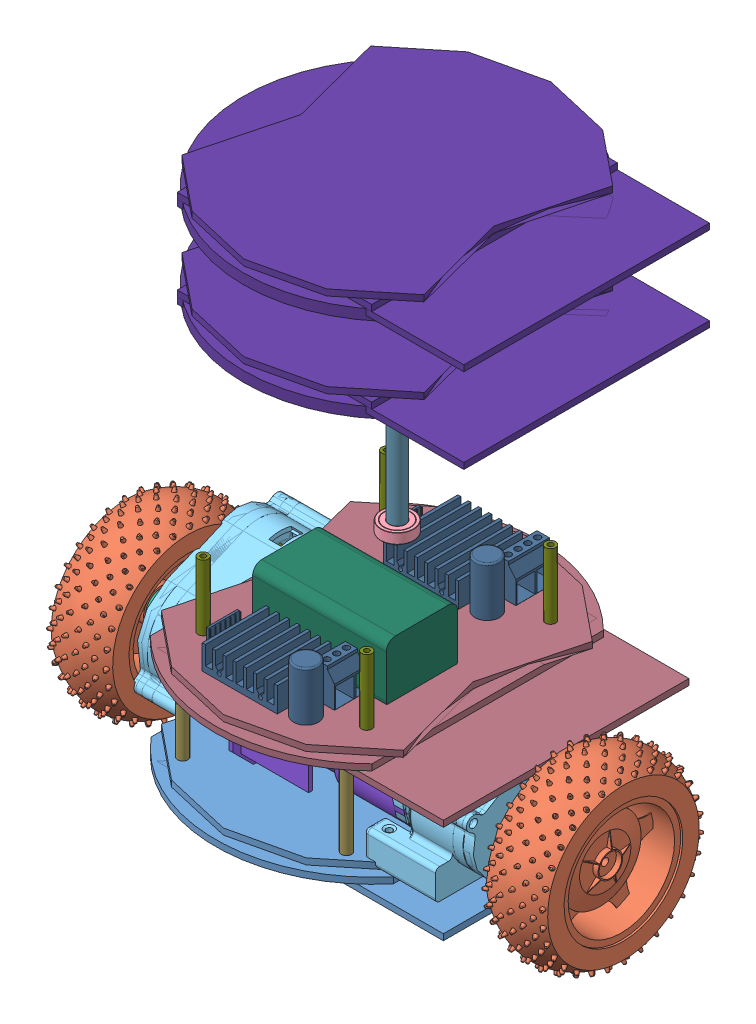
SolidWorks assembly Assembly_4, configuration Default. Lengths in mm.
Overall size (242.54 285.16 163.79).
38 component instances, 19 part files, 78 mates.
Components (placement in the parent):
- BASE PLATE COMPACT-1: BASE PLATE COMPACT [Default] at (9.1956 73.2306 176.3525) size (151.66 9 157.59)
- 85mm_Wheel-1: 85mm_Wheel [Default] at (-49.5434 86.804 117.1986) x (0 0.998679 -0.051377) z (0 0.051377 0.998679) size (89.76 30.03 89.76)
- Bearing_large-1: Bearing_large [Default] at (149.0346 86.804 117.1064) x (0 0.302035 0.953297) z (-1 0 0) size (34 34 10)
- Bearing_Modifiable-1: Bearing_Modifiable [Default] at (-9.2134 86.804 117.1986) x (0 0 -1) z (1 0 0) size (16 16 5)
- Gear Box Covering - Modifiable-1: Gear Box Covering - Modifiable [Default] at (122.6046 86.804 117.1064) x (0 -0.541121 -0.840945) z (1 0 0) size (87.3 57.46 46.55)
- Gear_Driven - LARGE-1: Gear_Driven - LARGE [Default] at (132.5346 86.804 117.1064) x (0 0.560889 0.827891) z (1 0 0) size (41.92 41.92 47.93)
- Gear_Driver-1: Gear_Driver [Default] at (129.4046 103.2 142.587) x (0 0.064546 -0.997915) z (1 0 0) size (21.81 21.81 25.3)
- IG32 MOTORS-1: IG32 MOTORS [Default] at (112.6046 103.2 142.587) x (-1 0 0) z (0 0 1) size (97 41 41.5)
- LINE SENSOR-1: LINE SENSOR [Default] at (106.6956 76.2306 130.3525) x (-1 0 0) z (0 0 1) size (100 13.5 28)
- Motor Driver-1: Motor Driver [Default] at (56.6226 127.2306 72.2216) x (0.999988 0 -0.00481) z (0.00481 0 0.999988) size (71 27 36.5)
- Motor_Main_Shaft-1: Motor_Main_Shaft [Default] at (112.6046 103.2 142.587) x (0 -0.924225 0.381849) z (1 0 0) size (6 6 15)
- Gear Box Covering - Modifiable-2: Gear Box Covering - Modifiable [Default] at (-9.2134 86.804 117.1986) x (0 -0.541121 0.840945) z (-1 0 0) size (87.3 57.46 46.55)
- IG32 MOTORS-2: IG32 MOTORS [Default] at (0.7866 103.2 91.718) size (97 41 41.5)
- Motor_Main_Shaft-2: Motor_Main_Shaft [Default] at (-14.2134 103.2 91.718) x (0 0 -1) z (1 0 0) size (6 6 15)
- Gear_Driver-2: Gear_Driver [Default] at (-16.0134 103.2 91.718) x (0 0.135257 0.99081) z (-1 0 0) size (21.81 21.81 25.3)
- Gear_Driven - LARGE-2: Gear_Driven - LARGE [Default] at (-19.1434 86.804 117.1986) x (0 0.998679 -0.051377) z (-1 0 0) size (41.92 41.92 47.93)
- Bearing_Modifiable-2: Bearing_Modifiable [Default] at (139.0346 103.2 142.587) x (0 -0.922949 -0.384923) z (1 0 0) size (16 16 5)
- Bearing_Modifiable-3: Bearing_Modifiable [Default] at (-30.6434 103.2 91.718) x (0 0.129255 -0.991611) z (1 0 0) size (16 16 5)
- Bearing_Modifiable-4: Bearing_Modifiable [Default] at (122.6046 86.804 117.1064) x (0 0.011286 0.999936) z (-1 0 0) size (16 16 5)
- Bearing_large-2: Bearing_large [Default] at (-35.6434 86.804 117.1986) x (0 0 -1) z (1 0 0) size (34 34 10)
- 85mm_Wheel-2: 85mm_Wheel [Default] at (162.9346 86.804 117.1064) x (0 -0.43653 0.89969) z (0 0.89969 0.43653) size (89.76 30.03 89.76)
- 4cm_spacers-1: 4cm_spacers [Default] at (96.6956 124.2306 61.5025) x (0.827993 0 0.560738) z (0 -1 0) size (5 5 50)
- 4cm_spacers-2: 4cm_spacers [Default] at (96.6956 124.2306 171.2025) x (0.889434 0 0.457064) z (0 -1 0) size (5 5 50)
- 4cm_spacers-3: 4cm_spacers [Default] at (16.6956 124.2306 171.2025) x (0.138561 0 0.990354) z (0 -1 0) size (5 5 50)
- 4cm_spacers-4: 4cm_spacers [Default] at (16.6956 124.2306 61.5025) x (0.594628 0 -0.804001) z (0 -1 0) size (5 5 50)
- Floor_Plates1-1: Floor_Plates1 [Default] at (9.1956 121.2306 176.3525) size (151.66 9 157.59)
- Motor Driver-2: Motor Driver [Default] at (56.6226 127.2306 160.7964) x (0.999988 0 -0.00481) z (0.00481 0 0.999988) size (71 27 36.5)
- Hex_Cover-1: Hex_Cover [Default] at (56.6956 76.2306 116.3525) x (0.996418 0 -0.084559) z (0.084559 0 0.996418) size (192.07 186 175) (hidden)
- Bearing_Modifiable-8: Bearing_Modifiable [Default] at (56.6956 170.2306 106.3525) x (0.129255 0 -0.991611) z (0 -1 0) size (16 16 5)
- Lead_Screw-1: Lead_Screw [Default] at (56.6956 165.2306 106.3525) size (7.8 140 7.8)
- BATTERY-1: BATTERY [Default] at (27.3177 127.2306 112.8472) x (0.999988 0 -0.00481) z (0.00481 0 0.999988) size (65 30 35)
- eYFi_Mega-1: eYFi_Mega [Default] at (54.6786 331.2306 173.9019) x (0.949338 0 -0.314256) z (0.314256 0 0.949338) size (150 18 150) (hidden)
- 3cm_spacers-6: 3cm_spacers [Default] at (16.6956 172.2306 71.5025) x (1 0 0) z (0 -1 0) size (5 5 40)
- 3cm_spacers-7: 3cm_spacers [Default] at (96.6956 172.2306 71.5025) x (1 0 0) z (0 -1 0) size (5 5 40)
- 3cm_spacers-9: 3cm_spacers [Default] at (96.6548 172.2306 161.2025) x (0.9912 0 0.132376) z (0 -1 0) size (5 5 40)
- 3cm_spacers-10: 3cm_spacers [Default] at (16.6956 172.2306 161.2025) x (0.967921 0 -0.251255) z (0 -1 0) size (5 5 40)
- Floor_Plates4_2-2: Floor_Plates4_2 [Default] at (9.1956 267.6556 166.3525) size (167.5 16 150)
- Floor_Plates4_2-3: Floor_Plates4_2 [Default] at (9.1956 309.0005 166.3525) size (167.5 16 150)
Mates (geometry in assembly coordinates):
- BasePlate_&_LineSensor: coincident anti-aligned: plane of BASE PLATE COMPACT-1 through (127.509 76.2306 116.3525) normal (0 -1 0); plane of LINE SENSOR-1 through (106.6956 76.2306 130.3525) normal (0 1 0)
- Potentiometer&BasePlate: parallel anti-aligned: plane of BASE PLATE COMPACT-1 through (29.6956 84.2306 121.8525) normal (-1 0 0); plane of LINE SENSOR-1 through (28.6956 81.2306 120.8525) normal (1 0 0)
- LineSensor&BasePlate: concentric anti-aligned: cylinder of BASE PLATE COMPACT-1 through (9.1956 84.2306 127.8525) axis (0 -1 0) radius 1.711; cylinder of LINE SENSOR-1 through (9.1956 74.2306 127.8525) axis (0 1 0) radius 1.5
- BasePlate&GearBox1: concentric aligned: cylinder of BASE PLATE COMPACT-1 through (4.0366 68.2306 132.1499) axis (0 1 0) radius 1.75; cylinder of Gear Box Covering - Modifiable-2 through (4.0366 67.8227 132.1499) axis (0 1 0) radius 1.75
- Coincident14: coincident anti-aligned: plane of BASE PLATE COMPACT-1 through (127.509 79.2306 116.3525) normal (0 1 0); plane of Gear Box Covering - Modifiable-2 through (-24.2134 79.2306 117.1986) normal (0 -1 0)
- GearBox&BasePlate1: parallel anti-aligned: plane of BASE PLATE COMPACT-1 through (-2.4644 76.2306 70.2538) normal (-1 0 0); plane of Gear Box Covering - Modifiable-2 through (-4.2134 103.2 91.718) normal (1 0 0)
- BasePlate&GearBox2: concentric aligned: cylinder of BASE PLATE COMPACT-1 through (109.3546 68.2306 102.1551) axis (0 1 0) radius 1.75; cylinder of Gear Box Covering - Modifiable-1 through (109.3546 67.8227 102.1551) axis (0 1 0) radius 1.75
- GearBox&BasePlate2: parallel anti-aligned: plane of BASE PLATE COMPACT-1 through (115.8556 76.2306 70.2538) normal (1 0 0); plane of Gear Box Covering - Modifiable-1 through (117.6046 103.2 142.587) normal (-1 0 0)
- BasePlate&GearBox2C: coincident anti-aligned: plane of BASE PLATE COMPACT-1 through (127.509 79.2306 116.3525) normal (0 1 0); plane of Gear Box Covering - Modifiable-1 through (137.6046 79.2306 117.1064) normal (0 -1 0)
- MotorShaft&GearBox2: concentric aligned: cylinder of IG32 MOTORS-1 through (115.6046 103.2 142.587) axis (-1 0 0) radius 7.5; cylinder of Motor_Main_Shaft-1 through (127.6046 103.2 142.587) axis (-1 0 0) radius 3
- Motor&MotorShaft2: coincident anti-aligned: plane of IG32 MOTORS-1 through (112.6046 103.2 142.587) normal (1 0 0); plane of Motor_Main_Shaft-1 through (112.6046 103.2 142.587) normal (-1 0 0)
- Motor&MotorShaft1: concentric anti-aligned: cylinder of IG32 MOTORS-2 through (-2.2134 103.2 91.718) axis (1 0 0) radius 7.5; cylinder of Motor_Main_Shaft-2 through (0.7866 103.2 91.718) axis (-1 0 0) radius 3
- Motor&MotorShaft11: coincident anti-aligned: plane of IG32 MOTORS-2 through (0.7866 103.2 91.718) normal (-1 0 0); plane of Motor_Main_Shaft-2 through (0.7866 103.2 91.718) normal (1 0 0)
- Motor&GearBox1: concentric aligned: cylinder of Gear Box Covering - Modifiable-2 through (-14.2134 103.2 91.718) axis (1 0 0) radius 10.75; cylinder of IG32 MOTORS-2 through (-2.2134 103.2 91.718) axis (1 0 0) radius 10.5
- Motor&GearBox2: concentric aligned: cylinder of Gear Box Covering - Modifiable-1 through (127.6046 103.2 142.587) axis (-1 0 0) radius 10.75; cylinder of IG32 MOTORS-1 through (115.6046 103.2 142.587) axis (-1 0 0) radius 10.5
- MotorHole&GearBox2: concentric aligned: cylinder of Gear Box Covering - Modifiable-1 through (117.6046 116.7 142.587) axis (1 0 0) radius 1.75; cylinder of IG32 MOTORS-1 through (109.6046 116.7 142.587) axis (1 0 0) radius 1.5
- MotorHole&GearBox1: concentric aligned: cylinder of Gear Box Covering - Modifiable-2 through (-4.2134 116.7 91.718) axis (-1 0 0) radius 1.75; cylinder of IG32 MOTORS-2 through (3.7866 116.7 91.718) axis (-1 0 0) radius 1.5
- Motor2&GearBox2: coincident anti-aligned: plane of Gear Box Covering - Modifiable-2 through (0.7866 103.2 91.718) normal (1 0 0); plane of IG32 MOTORS-2 through (0.7866 103.2 91.718) normal (-1 0 0)
- Motor1&GearBox1: coincident anti-aligned: plane of Gear Box Covering - Modifiable-1 through (112.6046 103.2 142.587) normal (-1 0 0); plane of IG32 MOTORS-1 through (112.6046 103.2 142.587) normal (1 0 0)
- Concentric17: concentric aligned: cylinder of Motor_Main_Shaft-2 through (0.7866 103.2 91.718) axis (-1 0 0) radius 3; cone of Gear_Driver-2 through (-4.2114 103.2 91.718) axis (-1 0 0)
- Coincident25: coincident anti-aligned: plane of Motor_Main_Shaft-2 through (-14.2134 103.2 91.718) normal (-1 0 0); plane of Gear_Driver-2 through (-14.2134 103.2 91.718) normal (1 0 0)
- Concentric18: concentric anti-aligned: cylinder of Gear_Driver-2 through (-16.5134 103.2 91.718) axis (-1 0 0) radius 2.8; cylinder of Bearing_Modifiable-3 through (-30.6434 103.2 91.718) axis (1 0 0) radius 8
- Coincident26: coincident aligned: plane of Gear Box Covering - Modifiable-2 through (-30.6434 109.5417 71.6985) normal (-1 0 0); plane of Bearing_Modifiable-3 through (-30.6434 103.2 91.718) normal (-1 0 0)
- Concentric20: concentric anti-aligned: cylinder of Gear_Driver-1 through (115.4046 103.2 142.587) axis (1 0 0) radius 5.75; cylinder of Motor_Main_Shaft-1 through (127.6046 103.2 142.587) axis (-1 0 0) radius 3
- Coincident27: coincident anti-aligned: plane of Gear_Driver-1 through (127.6046 103.2 142.587) normal (-1 0 0); plane of Motor_Main_Shaft-1 through (127.6046 103.2 142.587) normal (1 0 0)
- Concentric22: concentric aligned: cylinder of Gear_Driver-1 through (129.9046 103.2 142.587) axis (1 0 0) radius 2.8; cylinder of Bearing_Modifiable-2 through (139.0346 103.2 142.587) axis (1 0 0) radius 8
- Coincident28: coincident aligned: plane of Gear Box Covering - Modifiable-1 through (144.0346 109.5417 162.6066) normal (1 0 0); plane of Bearing_Modifiable-2 through (144.0346 103.2 142.587) normal (1 0 0)
- Concentric23: concentric anti-aligned: cylinder of Bearing_Modifiable-1 through (-9.2134 86.804 117.1986) axis (1 0 0) radius 8; cylinder of Gear Box Covering - Modifiable-2 through (-4.2134 86.804 117.1986) axis (-1 0 0) radius 8.75
- Coincident29: coincident aligned: plane of Bearing_Modifiable-1 through (-9.2134 86.804 117.1986) normal (-1 0 0); plane of Gear Box Covering - Modifiable-2 through (-9.2134 103.2 91.718) normal (-1 0 0)
- Concentric24: concentric anti-aligned: cylinder of Gear Box Covering - Modifiable-1 through (117.6046 86.804 117.1064) axis (1 0 0) radius 8.75; cylinder of Bearing_Modifiable-4 through (122.6046 86.804 117.1064) axis (-1 0 0) radius 8
- Coincident30: coincident aligned: plane of Gear Box Covering - Modifiable-1 through (122.6046 103.2 142.587) normal (1 0 0); plane of Bearing_Modifiable-4 through (122.6046 86.804 117.1064) normal (1 0 0)
- Concentric25: concentric aligned: cylinder of Bearing_Modifiable-1 through (-4.2134 86.804 117.1986) axis (-1 0 0) radius 3; cylinder of Gear_Driven - LARGE-2 through (-4.2134 86.804 117.1986) axis (-1 0 0) radius 2.8
- Coincident31: coincident anti-aligned: plane of Gear Box Covering - Modifiable-2 through (-4.2134 86.804 117.1986) normal (-1 0 0); plane of Gear_Driven - LARGE-2 through (-4.2134 86.804 117.1986) normal (1 0 0)
- Concentric26: concentric aligned: cylinder of Gear_Driven - LARGE-1 through (117.6046 86.804 117.1064) axis (1 0 0) radius 2.8; cylinder of Bearing_Modifiable-4 through (117.6046 86.804 117.1064) axis (1 0 0) radius 3
- Coincident32: coincident anti-aligned: plane of Gear Box Covering - Modifiable-1 through (117.6046 86.804 117.1064) normal (1 0 0); plane of Gear_Driven - LARGE-1 through (117.6046 86.804 117.1064) normal (-1 0 0)
- Concentric27: concentric anti-aligned: cylinder of Gear_Driven - LARGE-2 through (-47.9434 86.804 117.1986) axis (1 0 0) radius 7.5; cylinder of Bearing_large-2 through (-25.6434 86.804 117.1986) axis (-1 0 0) radius 7.5
- Concentric28: concentric anti-aligned: cylinder of Bearing_large-1 through (139.0346 86.804 117.1064) axis (1 0 0) radius 7.5; cylinder of Gear_Driven - LARGE-1 through (161.3346 86.804 117.1064) axis (-1 0 0) radius 7.5
- Coincident33: coincident aligned: plane of Gear Box Covering - Modifiable-2 through (-35.6434 86.804 117.1986) normal (-1 0 0); plane of Bearing_large-2 through (-35.6434 86.804 117.1986) normal (-1 0 0)
- Coincident34: coincident aligned: plane of Bearing_large-1 through (149.0346 86.804 117.1064) normal (1 0 0); plane of Gear Box Covering - Modifiable-1 through (149.0346 86.804 117.1064) normal (1 0 0)
- Concentric29: concentric anti-aligned: cylinder of 85mm_Wheel-1 through (-47.9434 86.804 117.1986) axis (-1 0 0) radius 8.5; cylinder of Gear_Driven - LARGE-2 through (-47.9434 86.804 117.1986) axis (1 0 0) radius 7.5
- Parallel1: parallel aligned: plane of 85mm_Wheel-1 through (-47.9434 92.6364 113.419) normal (0 -0.998679 0.051377); plane of Gear_Driven - LARGE-2 through (-52.1434 80.6145 114.0375) normal (0 -0.998679 0.051377)
- Coincident39: coincident anti-aligned: plane of 85mm_Wheel-1 through (-52.1434 86.804 117.1986) normal (1 0 0); plane of Gear_Driven - LARGE-2 through (-52.1434 86.804 117.1986) normal (-1 0 0)
- Concentric30: concentric anti-aligned: cylinder of Gear_Driven - LARGE-1 through (161.3346 86.804 117.1064) axis (-1 0 0) radius 7.5; cylinder of 85mm_Wheel-2 through (161.3346 86.804 117.1064) axis (1 0 0) radius 8.5
- Coincident41: coincident anti-aligned: plane of Gear_Driven - LARGE-1 through (165.5346 81.0502 121.0046) normal (0 -0.997419 0.071799); plane of 85mm_Wheel-2 through (161.3346 80.5511 114.0725) normal (0 0.997419 -0.071799)
- Coincident42: coincident anti-aligned: plane of Gear_Driven - LARGE-1 through (165.5346 86.804 117.1064) normal (1 0 0); plane of 85mm_Wheel-2 through (165.5346 86.804 117.1064) normal (-1 0 0)
- Concentric31: concentric anti-aligned: cylinder of BASE PLATE COMPACT-1 through (96.6956 86.2306 61.5025) axis (0 -1 0) radius 1.25; cylinder of 4cm_spacers-1 through (96.6956 74.2306 61.5025) axis (0 1 0) radius 1.25
- Coincident43: coincident anti-aligned: plane of BASE PLATE COMPACT-1 through (127.509 79.2306 116.3525) normal (0 1 0); plane of 4cm_spacers-1 through (96.6956 79.2306 61.5025) normal (0 -1 0)
- Concentric32: concentric anti-aligned: cylinder of BASE PLATE COMPACT-1 through (16.6956 86.2306 61.5025) axis (0 -1 0) radius 1.25; cylinder of 4cm_spacers-4 through (16.6956 74.2306 61.5025) axis (0 1 0) radius 1.25
- Concentric33: concentric anti-aligned: cylinder of BASE PLATE COMPACT-1 through (16.6956 86.2306 171.2025) axis (0 -1 0) radius 1.25; cylinder of 4cm_spacers-3 through (16.6956 74.2306 171.2025) axis (0 1 0) radius 1.25
- Concentric34: concentric anti-aligned: cylinder of BASE PLATE COMPACT-1 through (96.6956 86.2306 171.2025) axis (0 -1 0) radius 1.25; cylinder of 4cm_spacers-2 through (96.6956 74.2306 171.2025) axis (0 1 0) radius 1.25
- Coincident44: coincident anti-aligned: plane of BASE PLATE COMPACT-1 through (127.509 79.2306 116.3525) normal (0 1 0); plane of 4cm_spacers-4 through (16.6956 79.2306 61.5025) normal (0 -1 0)
- Coincident45: coincident anti-aligned: circle of BASE PLATE COMPACT-1; circle of 4cm_spacers-3
- Coincident46: coincident anti-aligned: plane of BASE PLATE COMPACT-1 through (127.509 79.2306 116.3525) normal (0 1 0); plane of 4cm_spacers-2 through (96.6956 79.2306 171.2025) normal (0 -1 0)
- Concentric35: concentric anti-aligned: cylinder of 4cm_spacers-4 through (16.6956 119.2306 61.5025) axis (0 1 0) radius 1.25; cylinder of Floor_Plates1-1 through (16.6956 134.2306 61.5025) axis (0 -1 0) radius 1.25
- Concentric36: concentric anti-aligned: line of 4cm_spacers-2 through (96.6956 119.2306 171.2025) axis (0 1 0); axis of Floor_Plates1-1 through (96.6956 127.2306 171.2025) axis (0 -1 0)
- Coincident47: coincident anti-aligned: plane of 4cm_spacers-1 through (96.6956 124.2306 61.5025) normal (0 1 0); plane of Floor_Plates1-1 through (127.509 124.2306 116.3525) normal (0 -1 0)
- Coincident48: coincident: plane of Floor_Plates1-1 through (127.509 127.2306 116.3525) normal (0 1 0); plane of Motor Driver-2 through (56.6226 127.2306 160.7964) normal (0 -1 0)
- Coincident49: coincident: plane of Motor Driver-1 through (56.6226 127.2306 72.2216) normal (0 -1 0); plane of Floor_Plates1-1 through (127.509 127.2306 116.3525) normal (0 1 0)
- Coincident64: coincident aligned: plane of BASE PLATE COMPACT-1 through (127.509 76.2306 116.3525) normal (0 -1 0); plane of Hex_Cover-1 through (56.6956 76.2306 116.3525) normal (0 -1 0)
- Coincident91: coincident: plane of Floor_Plates1-1 through (127.509 127.2306 116.3525) normal (0 1 0); plane of BATTERY-1 through (92.4853 127.2306 147.5341) normal (0 -1 0)
- Parallel2: parallel aligned: plane of Motor Driver-2 through (92.21 129.2306 178.8754) normal (0.999988 0 -0.00481); plane of BATTERY-1 through (92.4853 157.2306 147.5341) normal (0.999988 0 -0.00481)
- Coincident94: coincident: plane of Motor Driver-2 through (92.21 129.2306 178.8754) normal (0.999988 0 -0.00481); plane of BATTERY-1 through (92.4853 157.2306 147.5341) normal (0.999988 0 -0.00481)
- Coincident95: coincident: plane of Motor Driver-1 through (92.21 129.2306 90.3007) normal (0.999988 0 -0.00481); plane of BATTERY-1 through (92.4853 157.2306 147.5341) normal (0.999988 0 -0.00481)
- Concentric88: concentric: cylinder of Floor_Plates1-1 through (89.1956 134.2306 175.8899) axis (0 -1 0) radius 1.5; cylinder of Motor Driver-2 through (89.1956 127.2306 175.8899) axis (0 1 0) radius 1.5
- Concentric89: concentric: cylinder of Floor_Plates1-1 through (24.1956 134.2306 176.2025) axis (0 -1 0) radius 1.5; cylinder of Motor Driver-2 through (24.1963 127.2306 176.2025) axis (0 1 0) radius 1.5
- Concentric93: concentric: cylinder of Motor Driver-1 through (89.1956 127.2306 87.3152) axis (0 1 0) radius 1.5; cylinder of Floor_Plates1-1 through (89.1956 134.2306 87.3152) axis (0 -1 0) radius 1.5
- Concentric96: concentric anti-aligned: cylinder of Floor_Plates1-1 through (96.6956 134.2306 71.5025) axis (0 -1 0) radius 1.5; cylinder of 3cm_spacers-7 through (96.6956 122.2306 71.5025) axis (0 1 0) radius 1.25
- Concentric97: concentric anti-aligned: cylinder of Floor_Plates1-1 through (16.6956 134.2306 71.5025) axis (0 -1 0) radius 1.5; cylinder of 3cm_spacers-6 through (16.6956 122.2306 71.5025) axis (0 1 0) radius 1.25
- Coincident109: coincident anti-aligned: plane of Floor_Plates1-1 through (127.509 127.2306 116.3525) normal (0 1 0); plane of 3cm_spacers-6 through (16.6956 127.2306 71.5025) normal (0 -1 0)
- Coincident112: coincident anti-aligned: plane of Floor_Plates1-1 through (127.509 127.2306 116.3525) normal (0 1 0); plane of 3cm_spacers-7 through (96.6956 127.2306 71.5025) normal (0 -1 0)
- Concentric98: concentric anti-aligned: cylinder of Floor_Plates1-1 through (16.6956 134.2306 161.2025) axis (0 -1 0) radius 1.5; cylinder of 3cm_spacers-10 through (16.6956 122.2306 161.2025) axis (0 1 0) radius 1.25
- Concentric99: concentric anti-aligned: cylinder of Floor_Plates1-1 through (96.6548 134.2306 161.2025) axis (0 -1 0) radius 1.5; cylinder of 3cm_spacers-9 through (96.6548 122.2306 161.2025) axis (0 1 0) radius 1.25
- Coincident113: coincident anti-aligned: plane of Floor_Plates1-1 through (127.509 127.2306 116.3525) normal (0 1 0); plane of 3cm_spacers-9 through (96.6548 127.2306 161.2025) normal (0 -1 0)
- Coincident114: coincident anti-aligned: plane of Floor_Plates1-1 through (127.509 127.2306 116.3525) normal (0 1 0); plane of 3cm_spacers-10 through (16.6956 127.2306 161.2025) normal (0 -1 0)
- Concentric102: concentric anti-aligned: cylinder of Bearing_Modifiable-8 through (56.6956 165.2306 106.3525) axis (0 1 0) radius 3; cylinder of Lead_Screw-1 through (56.6956 305.2306 106.3525) axis (0 -1 0) radius 3.9
- Concentric103: concentric anti-aligned: cylinder of Lead_Screw-1 through (56.6956 305.2306 106.3525) axis (0 -1 0) radius 3.9; cylinder of Floor_Plates4_2-2 through (56.6956 260.6556 106.3525) axis (0 1 0) radius 8.5
- Concentric104: concentric aligned: cylinder of Floor_Plates4_2-2 through (56.6956 260.6556 106.3525) axis (0 1 0) radius 8.5; cylinder of Floor_Plates4_2-3 through (56.6956 302.0005 106.3525) axis (0 1 0) radius 8.5
- Concentric105: concentric aligned: cylinder of Floor_Plates4_2-2 through (116.6956 260.6556 106.3525) axis (0 1 0) radius 8.5; cylinder of Floor_Plates4_2-3 through (116.6956 302.0005 106.3525) axis (0 1 0) radius 8.5
